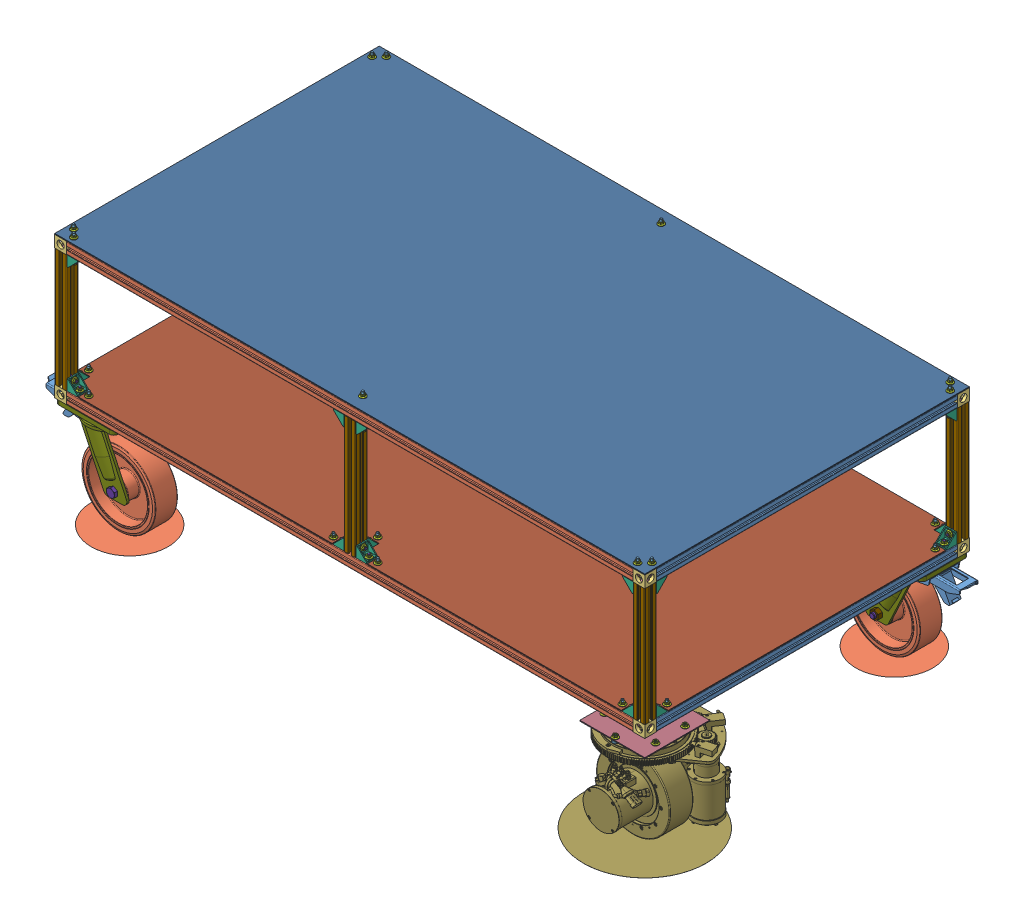
SolidWorks assembly totale, configuration Default. Lengths in mm. (continued)
Components (placement in the parent): (continued)
- body-1: body [Default] at (-233.7628 101.484 2240) size (2000 498.7 1100) (continued)
  - body_skeleton-1: body_skeleton [Default] at (-1.581 -195.357 0) size (2000 480 1100) (continued)
    - Piano_base-2: Piano_base [Default] at (1030.9122 410.7283 -1270) x (1 0 0) z (0 0 -1) size (2000 66.8 1100) (continued)
      - longherone_h-6: longherone_h [Default] at (-560.5014 -11.1801 -790) size (112 40 1043.4)
        - profilato_1020-1: profilato_1020 [Default] at (33.8348 -8.8199 -750) size (40 40 1020)
        - T_BOLT-1: T_BOLT [Default] at (33.8348 -8.8199 276) x (0 -1 0) z (0 0 1) size (19.4 8.5 30.4)
        - T_BOLT-2: T_BOLT [Default] at (33.8348 -8.8199 -756) x (0 -1 0) z (0 0 -1) size (19.4 8.5 30.4)
        - Bracket_40_40_set-2: Bracket_40_40_set [Default] at (-7.7665 -12.3804 -732) x (0 1 0) z (0 0 1) size (38 47.7 51.56)
          - bracket_40_40-1: bracket_40_40 [Default] at (-15.4395 -1.6013 2) size (38 36 36)
          - FLANGE_NUT_M8-3: FLANGE_NUT_M8 [Default] at (3.5605 3.5487 -12.5) size (21 21 8)
          - T_BOLT_short-4: T_BOLT_short [Default] at (3.5605 3.5487 -24) x (-1 0 0) z (0 0 -1) size (19.4 8.5 26.9)
          - FLANGE_NUT_M8-4: FLANGE_NUT_M8 [Default] at (3.5605 -16.1013 7.15) x (0.797177 0 0.603746) z (0 1 0) size (21 21 8)
          - T_BOLT_short-5: T_BOLT_short [Default] at (3.5605 -27.6013 7.15) x (-1 0 0) z (0 -1 0) size (19.4 8.5 26.9)
        - Bracket_40_40_set-3: Bracket_40_40_set [Default] at (75.436 -5.2593 -732) x (0 -1 0) z (0 0 1) size (38 47.7 51.56)
          - bracket_40_40-1: bracket_40_40 [Default] at (-15.4395 -1.6013 2) size (38 36 36)
          - FLANGE_NUT_M8-3: FLANGE_NUT_M8 [Default] at (3.5605 3.5487 -12.5) size (21 21 8)
          - T_BOLT_short-4: T_BOLT_short [Default] at (3.5605 3.5487 -24) x (-1 0 0) z (0 0 -1) size (19.4 8.5 26.9)
          - FLANGE_NUT_M8-4: FLANGE_NUT_M8 [Default] at (3.5605 -16.1013 7.15) x (0.797177 0 0.603746) z (0 1 0) size (21 21 8)
          - T_BOLT_short-5: T_BOLT_short [Default] at (3.5605 -27.6013 7.15) x (-1 0 0) z (0 -1 0) size (19.4 8.5 26.9)
        - Bracket_40_40_set-4: Bracket_40_40_set [Default] at (75.436 -12.3804 252) x (0 1 0) z (0 0 -1) size (38 47.7 51.56)
          - bracket_40_40-1: bracket_40_40 [Default] at (-15.4395 -1.6013 2) size (38 36 36)
          - FLANGE_NUT_M8-3: FLANGE_NUT_M8 [Default] at (3.5605 3.5487 -12.5) size (21 21 8)
          - T_BOLT_short-4: T_BOLT_short [Default] at (3.5605 3.5487 -24) x (-1 0 0) z (0 0 -1) size (19.4 8.5 26.9)
          - FLANGE_NUT_M8-4: FLANGE_NUT_M8 [Default] at (3.5605 -16.1013 7.15) x (0.797177 0 0.603746) z (0 1 0) size (21 21 8)
          - T_BOLT_short-5: T_BOLT_short [Default] at (3.5605 -27.6013 7.15) x (-1 0 0) z (0 -1 0) size (19.4 8.5 26.9)
        - Bracket_40_40_set-5: Bracket_40_40_set [Default] at (-7.7665 -5.2593 252) x (0 -1 0) z (0 0 -1) size (38 47.7 51.56)
          - bracket_40_40-1: bracket_40_40 [Default] at (-15.4395 -1.6013 2) size (38 36 36)
          - FLANGE_NUT_M8-3: FLANGE_NUT_M8 [Default] at (3.5605 3.5487 -12.5) size (21 21 8)
          - T_BOLT_short-4: T_BOLT_short [Default] at (3.5605 3.5487 -24) x (-1 0 0) z (0 0 -1) size (19.4 8.5 26.9)
          - FLANGE_NUT_M8-4: FLANGE_NUT_M8 [Default] at (3.5605 -16.1013 7.15) x (0.797177 0 0.603746) z (0 1 0) size (21 21 8)
          - T_BOLT_short-5: T_BOLT_short [Default] at (3.5605 -27.6013 7.15) x (-1 0 0) z (0 -1 0) size (19.4 8.5 26.9)
      - Bracket_40_40_set-1: Bracket_40_40_set [Default] at (-58 -23.5605 -541.6013) x (0 1 0) z (-1 0 0) size (38 47.7 51.56)
        - bracket_40_40-1: bracket_40_40 [Default] at (-15.4395 -1.6013 2) size (38 36 36)
        - FLANGE_NUT_M8-3: FLANGE_NUT_M8 [Default] at (3.5605 3.5487 -12.5) size (21 21 8)
        - T_BOLT_short-4: T_BOLT_short [Default] at (3.5605 3.5487 -24) x (-1 0 0) z (0 0 -1) size (19.4 8.5 26.9)
        - FLANGE_NUT_M8-4: FLANGE_NUT_M8 [Default] at (3.5605 -16.1013 7.15) x (0.797177 0 0.603746) z (0 1 0) size (21 21 8)
        - T_BOLT_short-5: T_BOLT_short [Default] at (3.5605 -27.6013 7.15) x (-1 0 0) z (0 -1 0) size (19.4 8.5 26.9)
      - Bracket_40_40_set-2: Bracket_40_40_set [Default] at (-1942 -16.4395 -541.6013) x (0 -1 0) z (1 0 0) size (38 47.7 51.56)
        - bracket_40_40-1: bracket_40_40 [Default] at (-15.4395 -1.6013 2) size (38 36 36)
        - FLANGE_NUT_M8-3: FLANGE_NUT_M8 [Default] at (3.5605 3.5487 -12.5) size (21 21 8)
        - T_BOLT_short-4: T_BOLT_short [Default] at (3.5605 3.5487 -24) x (-1 0 0) z (0 0 -1) size (19.4 8.5 26.9)
        - FLANGE_NUT_M8-4: FLANGE_NUT_M8 [Default] at (3.5605 -16.1013 7.15) x (0.797177 0 0.603746) z (0 1 0) size (21 21 8)
        - T_BOLT_short-5: T_BOLT_short [Default] at (3.5605 -27.6013 7.15) x (-1 0 0) z (0 -1 0) size (19.4 8.5 26.9)
      - Bracket_40_40_set-3: Bracket_40_40_set [Default] at (-58 -16.4395 -1518.3987) x (0 -1 0) z (-1 0 0) size (38 47.7 51.56)
        - bracket_40_40-1: bracket_40_40 [Default] at (-15.4395 -1.6013 2) size (38 36 36)
        - FLANGE_NUT_M8-3: FLANGE_NUT_M8 [Default] at (3.5605 3.5487 -12.5) size (21 21 8)
        - T_BOLT_short-4: T_BOLT_short [Default] at (3.5605 3.5487 -24) x (-1 0 0) z (0 0 -1) size (19.4 8.5 26.9)
        - FLANGE_NUT_M8-4: FLANGE_NUT_M8 [Default] at (3.5605 -16.1013 7.15) x (0.797177 0 0.603746) z (0 1 0) size (21 21 8)
        - T_BOLT_short-5: T_BOLT_short [Default] at (3.5605 -27.6013 7.15) x (-1 0 0) z (0 -1 0) size (19.4 8.5 26.9)
      - Bracket_40_40_set-4: Bracket_40_40_set [Default] at (-1938.3987 -16.4395 -1522) x (0 -1 0) z (0 0 1) size (38 47.7 51.56)
        - bracket_40_40-1: bracket_40_40 [Default] at (-15.4395 -1.6013 2) size (38 36 36)
        - FLANGE_NUT_M8-3: FLANGE_NUT_M8 [Default] at (3.5605 3.5487 -12.5) size (21 21 8)
        - T_BOLT_short-4: T_BOLT_short [Default] at (3.5605 3.5487 -24) x (-1 0 0) z (0 0 -1) size (19.4 8.5 26.9)
        - FLANGE_NUT_M8-4: FLANGE_NUT_M8 [Default] at (3.5605 -16.1013 7.15) x (0.797177 0 0.603746) z (0 1 0) size (21 21 8)
        - T_BOLT_short-5: T_BOLT_short [Default] at (3.5605 -27.6013 7.15) x (-1 0 0) z (0 -1 0) size (19.4 8.5 26.9)
  - lastra-1: lastra [Default] at (29.3311 258.3712 -240) x (0 0 1) z (0 1 0) size (1100 2000 3)
  - lastra_down-1: lastra_down [Default] at (29.3311 -184.6288 -240) x (0 0 -1) z (0 -1 0) size (1100 2000 3)
  - T_BOLT-1: T_BOLT [Default] at (-950.6689 -190.6288 -694.75) x (1 0 0) z (0 -1 0) size (19.4 8.5 30.4)
  - T_BOLT-2: T_BOLT [Default] at (-875.4189 -190.6288 -770) x (0 0 1) z (0 -1 0) size (19.4 8.5 30.4)
  - T_BOLT-3: T_BOLT [Default] at (-950.6689 -190.6288 214.75) x (1 0 0) z (0 -1 0) size (19.4 8.5 30.4)
  - T_BOLT-4: T_BOLT [Default] at (-875.4189 -190.6288 290) x (0 0 -1) z (0 -1 0) size (19.4 8.5 30.4)
  - T_BOLT-5: T_BOLT [Default] at (-950.6689 249.3712 -745.75) x (-1 0 0) z (0 -1 0) size (19.4 8.5 30.4)
  - T_BOLT-6: T_BOLT [Default] at (-926.4189 249.3712 -770) x (0 0 -1) z (0 -1 0) size (19.4 8.5 30.4)
  - T_BOLT-7: T_BOLT [Default] at (985.0811 249.3712 -770) x (0 0 -1) z (0 -1 0) size (19.4 8.5 30.4)
  - T_BOLT-8: T_BOLT [Default] at (1009.3311 249.3712 -745.75) x (-1 0 0) z (0 -1 0) size (19.4 8.5 30.4)
  - T_BOLT-9: T_BOLT [Default] at (1009.3311 -190.6288 -694.75) x (-1 0 0) z (0 -1 0) size (19.4 8.5 30.4)
  - T_BOLT-10: T_BOLT [Default] at (934.0811 -190.6288 -770) x (0 0 -1) z (0 -1 0) size (19.4 8.5 30.4)
  - T_BOLT-11: T_BOLT [Default] at (985.0811 249.3712 290) x (0 0 -1) z (0 -1 0) size (19.4 8.5 30.4)
  - T_BOLT-12: T_BOLT [Default] at (1009.3311 249.3712 265.75) x (1 0 0) z (0 -1 0) size (19.4 8.5 30.4)
  - T_BOLT-13: T_BOLT [Default] at (934.0811 -190.6288 290) x (0 0 -1) z (0 -1 0) size (19.4 8.5 30.4)
  - T_BOLT-14: T_BOLT [Default] at (1009.3311 -190.6288 214.75) x (1 0 0) z (0 -1 0) size (19.4 8.5 30.4)
  - T_BOLT-15: T_BOLT [Default] at (-45.9189 -190.6288 290) x (0 0 -1) z (0 -1 0) size (19.4 8.5 30.4)
  - T_BOLT-16: T_BOLT [Default] at (104.5811 -190.6288 290) x (0 0 1) z (0 -1 0) size (19.4 8.5 30.4)
  - T_BOLT-17: T_BOLT [Default] at (29.3311 -190.6288 -694.75) x (-1 0 0) z (0 -1 0) size (19.4 8.5 30.4)
  - T_BOLT-18: T_BOLT [Default] at (-950.6689 249.3712 265.75) x (1 0 0) z (0 -1 0) size (19.4 8.5 30.4)
  - T_BOLT-19: T_BOLT [Default] at (-45.9189 -190.6288 -770) x (0 0 -1) z (0 -1 0) size (19.4 8.5 30.4)
  - T_BOLT-20: T_BOLT [Default] at (104.5811 -190.6288 -770) x (0 0 1) z (0 -1 0) size (19.4 8.5 30.4)
  - T_BOLT-21: T_BOLT [Default] at (29.3311 249.3712 -745.75) x (-1 0 0) z (0 -1 0) size (19.4 8.5 30.4)
  - T_BOLT-22: T_BOLT [Default] at (29.3311 -190.6288 214.75) x (1 0 0) z (0 -1 0) size (19.4 8.5 30.4)
  - T_BOLT-23: T_BOLT [Default] at (29.3311 249.3712 265.75) x (-1 0 0) z (0 -1 0) size (19.4 8.5 30.4)
  - T_BOLT-24: T_BOLT [Default] at (-926.4189 249.3712 290) x (0 0 -1) z (0 -1 0) size (19.4 8.5 30.4)
  - FLANGE_NUT_M8-1: FLANGE_NUT_M8 [Default] at (-950.6689 -181.6288 -694.75) x (1 0 0) z (0 1 0) size (21 21 8)
  - FLANGE_NUT_M8-2: FLANGE_NUT_M8 [Default] at (29.3311 258.3712 -745.75) x (0.999686 0 0.025076) z (0 1 0) size (21 21 8)
  - FLANGE_NUT_M8-3: FLANGE_NUT_M8 [Default] at (29.3311 -181.6288 -694.75) x (1 0 0) z (0 1 0) size (21 21 8)
  - FLANGE_NUT_M8-4: FLANGE_NUT_M8 [Default] at (-875.4189 -181.6288 -770) x (1 0 0) z (0 1 0) size (21 21 8)
  - FLANGE_NUT_M8-5: FLANGE_NUT_M8 [Default] at (-875.4189 -181.6288 290) x (1 0 0) z (0 1 0) size (21 21 8)
  - FLANGE_NUT_M8-6: FLANGE_NUT_M8 [Default] at (-950.6689 -181.6288 214.75) x (1 0 0) z (0 1 0) size (21 21 8)
  - FLANGE_NUT_M8-7: FLANGE_NUT_M8 [Default] at (-45.9189 -181.6288 -770) x (1 0 0) z (0 1 0) size (21 21 8)
  - FLANGE_NUT_M8-8: FLANGE_NUT_M8 [Default] at (-45.9189 -181.6288 290) x (1 0 0) z (0 1 0) size (21 21 8)
  - FLANGE_NUT_M8-9: FLANGE_NUT_M8 [Default] at (-950.6689 258.3712 -745.75) x (1 0 0) z (0 1 0) size (21 21 8)
  - FLANGE_NUT_M8-10: FLANGE_NUT_M8 [Default] at (985.0811 258.3712 -770) x (1 0 0) z (0 1 0) size (21 21 8)
  - FLANGE_NUT_M8-11: FLANGE_NUT_M8 [Default] at (-926.4189 258.3712 290) x (1 0 0) z (0 1 0) size (21 21 8)
  - FLANGE_NUT_M8-12: FLANGE_NUT_M8 [Default] at (1009.3311 258.3712 -745.75) x (1 0 0) z (0 1 0) size (21 21 8)
  - FLANGE_NUT_M8-13: FLANGE_NUT_M8 [Default] at (1009.3311 258.3712 265.75) x (1 0 0) z (0 1 0) size (21 21 8)
  - FLANGE_NUT_M8-14: FLANGE_NUT_M8 [Default] at (934.0811 -181.6288 290) x (1 0 0) z (0 1 0) size (21 21 8)
  - FLANGE_NUT_M8-15: FLANGE_NUT_M8 [Default] at (-926.4189 258.3712 -770) x (1 0 0) z (0 1 0) size (21 21 8)
  - FLANGE_NUT_M8-16: FLANGE_NUT_M8 [Default] at (29.3311 -181.6288 214.75) x (1 0 0) z (0 1 0) size (21 21 8)
  - FLANGE_NUT_M8-17: FLANGE_NUT_M8 [Default] at (934.0811 -181.6288 -770) x (1 0 0) z (0 1 0) size (21 21 8)
  - FLANGE_NUT_M8-18: FLANGE_NUT_M8 [Default] at (104.5811 -181.6288 -770) x (1 0 0) z (0 1 0) size (21 21 8)
  - FLANGE_NUT_M8-19: FLANGE_NUT_M8 [Default] at (1009.3311 -181.6288 214.75) x (1 0 0) z (0 1 0) size (21 21 8)
  - FLANGE_NUT_M8-20: FLANGE_NUT_M8 [Default] at (-950.6689 258.3712 265.75) x (1 0 0) z (0 1 0) size (21 21 8)
  - FLANGE_NUT_M8-21: FLANGE_NUT_M8 [Default] at (985.0811 258.3712 290) x (1 0 0) z (0 1 0) size (21 21 8)
  - FLANGE_NUT_M8-22: FLANGE_NUT_M8 [Default] at (104.5811 -181.6288 290) x (1 0 0) z (0 1 0) size (21 21 8)
  - FLANGE_NUT_M8-23: FLANGE_NUT_M8 [Default] at (1009.3311 -181.6288 -694.75) x (1 0 0) z (0 1 0) size (21 21 8)
  - FLANGE_NUT_M8-24: FLANGE_NUT_M8 [Default] at (29.3311 258.3712 265.75) x (1 0 0) z (0 1 0) size (21 21 8)
- motore+supporto-1: motore+supporto [Default] at (-1125.506 -711.9473 1513.7207) x (-0.999869 -0.016207 0) z (-0.016207 0.999869 -0.000006) size (415.84 415.9 330.44)
  - MR240FRS-AC.stp-1: MR240FRS-AC.stp [Default] at (480.9296 100.5307 -916.9118) size (415.84 415.9 312.91)
  - supporto_motore-2: supporto_motore [Default] at (5.5916 0.2825 575.9688) x (-0.999869 0 -0.016207) z (0.016207 -0.000006 -0.999869) size (220 220 3)
  - distanziale-1: distanziale [Default] at (92.3448 50.2824 567.3735) x (0.92025 -0.391047 0.014919) z (-0.016207 0.000006 0.999869) size (18 18 10)
  - distanziale-2: distanziale [Default] at (-80.8375 -49.7176 564.5668) x (-0.654362 0.756107 -0.010611) z (-0.016207 0.000006 0.999869) size (18 18 10)
  - distanziale-3: distanziale [Default] at (5.7536 -99.7176 565.9707) x (-0.654362 0.756107 -0.010611) z (-0.016207 0.000006 0.999869) size (18 18 10)
  - distanziale-4: distanziale [Default] at (5.5916 100.2825 575.9683) x (-0.701568 -0.712512 -0.011368) z (0.016207 -0.000006 -0.999869) size (18 18 10)
  - distanziale-5: distanziale [Default] at (92.3448 -49.7176 567.374) x (-0.654362 0.756107 -0.010611) z (-0.016207 0.000006 0.999869) size (18 18 10)
  - distanziale-6: distanziale [Default] at (-80.8375 50.2824 564.5663) x (0.92025 -0.391047 0.014919) z (-0.016207 0.000006 0.999869) size (18 18 10)
  - distanziale-7: distanziale [Default] at (-28.6146 -43.7175 588.4163) x (0.316566 0.948557 0.005126) z (0.016207 -0.000006 -0.999869) size (18 18 10)
  - distanziale-8: distanziale [Default] at (49.3751 34.2825 589.6801) x (0.316566 0.948557 0.005126) z (0.016207 -0.000006 -0.999869) size (18 18 10)
  - distanziale-9: distanziale [Default] at (25.1283 -43.7175 589.2875) x (-0.701568 -0.712512 -0.011368) z (0.016207 -0.000006 -0.999869) size (18 18 10)
  - FLANGE_NUT_M8-1: FLANGE_NUT_M8 [Default] at (92.1341 -49.7175 580.3723) x (0.999869 0 0.016207) z (-0.016207 0.000006 0.999869) size (21 21 8)
  - FLANGE_NUT_M8-2: FLANGE_NUT_M8 [Default] at (-81.0482 50.2825 577.5646) x (0.999869 0 0.016207) z (-0.016207 0.000006 0.999869) size (21 21 8)
  - FLANGE_NUT_M8-3: FLANGE_NUT_M8 [Default] at (-81.0482 -49.7175 577.5651) x (0.999869 0 0.016207) z (-0.016207 0.000006 0.999869) size (21 21 8)
  - FLANGE_NUT_M8-4: FLANGE_NUT_M8 [Default] at (5.5429 -99.7175 578.969) x (0.999869 0 0.016207) z (-0.016207 0.000006 0.999869) size (21 21 8)
  - FLANGE_NUT_M8-5: FLANGE_NUT_M8 [Default] at (5.543 100.2825 578.9679) x (0.999869 0 0.016207) z (-0.016207 0.000006 0.999869) size (21 21 8)
  - FLANGE_NUT_M8-6: FLANGE_NUT_M8 [Default] at (92.1342 50.2825 580.3717) x (0.999869 0 0.016207) z (-0.016207 0.000006 0.999869) size (21 21 8)
  - FLANGE_NUT_M8-7: FLANGE_NUT_M8 [Default] at (-28.4039 -43.7175 575.418) x (-0.924292 -0.381392 -0.01498) z (0.016207 -0.000006 -0.999869) size (21 21 8)
  - FLANGE_NUT_M8-8: FLANGE_NUT_M8 [Default] at (25.339 -43.7175 576.2892) x (0.999868 -0.000687 0.016207) z (0.016207 -0.000006 -0.999869) size (21 21 8)
  - FLANGE_NUT_M8-9: FLANGE_NUT_M8 [Default] at (49.5858 34.2825 576.6818) x (-0.924292 -0.381392 -0.01498) z (0.016207 -0.000006 -0.999869) size (21 21 8)
  - slotted countersunk flat head screw_iso-1: slotted countersunk flat head screw_iso [ISO 2009 - M8 x 50 - 38N] at (-80.3351 -49.7178 533.5709) x (-0.016207 0.000006 0.999869) z (-0.999869 -0.000006 -0.016207) size (50 15.8 15.67)
  - slotted countersunk flat head screw_iso-2: slotted countersunk flat head screw_iso [ISO 2009 - M8 x 50 - 38N] at (-3.804 -13.9391 527.2162) size (50 15.8 15.67)
  - slotted countersunk flat head screw_iso-4: slotted countersunk flat head screw_iso [ISO 2009 - M8 x 50 - 38N] at (6.2561 -99.7178 534.9748) x (-0.016207 0.000006 0.999869) z (-0.999869 -0.000006 -0.016207) size (50 15.8 15.67)
  - slotted countersunk flat head screw_iso-5: slotted countersunk flat head screw_iso [ISO 2009 - M8 x 50 - 38N] at (92.8472 -49.7178 536.3781) x (-0.016207 0.000006 0.999869) z (-0.999869 -0.000006 -0.016207) size (50 15.8 15.67)
  - slotted countersunk flat head screw_iso-6: slotted countersunk flat head screw_iso [ISO 2009 - M8 x 50 - 38N] at (-80.3351 50.2822 533.5704) x (-0.016207 0.000006 0.999869) z (-0.999869 -0.000006 -0.016207) size (50 15.8 15.67)
  - slotted countersunk flat head screw_iso-7: slotted countersunk flat head screw_iso [ISO 2009 - M8 x 50 - 38N] at (6.2561 100.2822 534.9737) x (-0.016207 0.000006 0.999869) z (-0.999869 -0.000006 -0.016207) size (50 15.8 15.67)
  - slotted countersunk flat head screw_iso-8: slotted countersunk flat head screw_iso [ISO 2009 - M8 x 50 - 38N] at (92.8473 50.2822 536.3775) x (-0.016207 0.000006 0.999869) z (-0.999869 -0.000006 -0.016207) size (50 15.8 15.67)
  - distanziale-10: distanziale [Default] at (49.3751 -19.4675 589.6804) x (-0.807591 -0.589598 -0.013087) z (0.016207 -0.000006 -0.999869) size (18 18 10)
  - FLANGE_NUT_M8-10: FLANGE_NUT_M8 [Default] at (49.5858 -19.4675 576.6821) x (-0.924292 -0.381392 -0.01498) z (0.016207 -0.000006 -0.999869) size (21 21 8)
- motore+supporto-2: motore+supporto [Default] at (716.6426 -711.9473 2486.2793) x (0.999869 -0.016207 0) z (0.016207 0.999869 0.000006) size (415.84 415.9 330.44)
  - MR240FRS-AC.stp-1: MR240FRS-AC.stp [Default] at (480.9296 100.5307 -916.9118) size (415.84 415.9 312.91)
  - supporto_motore-2: supporto_motore [Default] at (5.5916 0.2825 575.9688) x (-0.999869 0 -0.016207) z (0.016207 -0.000006 -0.999869) size (220 220 3)
  - distanziale-1: distanziale [Default] at (92.3448 50.2824 567.3735) x (0.92025 -0.391047 0.014919) z (-0.016207 0.000006 0.999869) size (18 18 10)
  - distanziale-2: distanziale [Default] at (-80.8375 -49.7176 564.5668) x (-0.654362 0.756107 -0.010611) z (-0.016207 0.000006 0.999869) size (18 18 10)
  - distanziale-3: distanziale [Default] at (5.7536 -99.7176 565.9707) x (-0.654362 0.756107 -0.010611) z (-0.016207 0.000006 0.999869) size (18 18 10)
  - distanziale-4: distanziale [Default] at (5.5916 100.2825 575.9683) x (-0.701568 -0.712512 -0.011368) z (0.016207 -0.000006 -0.999869) size (18 18 10)
  - distanziale-5: distanziale [Default] at (92.3448 -49.7176 567.374) x (-0.654362 0.756107 -0.010611) z (-0.016207 0.000006 0.999869) size (18 18 10)
  - distanziale-6: distanziale [Default] at (-80.8375 50.2824 564.5663) x (0.92025 -0.391047 0.014919) z (-0.016207 0.000006 0.999869) size (18 18 10)
  - distanziale-7: distanziale [Default] at (-28.6146 -43.7175 588.4163) x (0.316566 0.948557 0.005126) z (0.016207 -0.000006 -0.999869) size (18 18 10)
  - distanziale-8: distanziale [Default] at (49.3751 34.2825 589.6801) x (0.316566 0.948557 0.005126) z (0.016207 -0.000006 -0.999869) size (18 18 10)
  - distanziale-9: distanziale [Default] at (25.1283 -43.7175 589.2875) x (-0.701568 -0.712512 -0.011368) z (0.016207 -0.000006 -0.999869) size (18 18 10)
  - FLANGE_NUT_M8-1: FLANGE_NUT_M8 [Default] at (92.1341 -49.7175 580.3723) x (0.999869 0 0.016207) z (-0.016207 0.000006 0.999869) size (21 21 8)
  - FLANGE_NUT_M8-2: FLANGE_NUT_M8 [Default] at (-81.0482 50.2825 577.5646) x (0.999869 0 0.016207) z (-0.016207 0.000006 0.999869) size (21 21 8)
  - FLANGE_NUT_M8-3: FLANGE_NUT_M8 [Default] at (-81.0482 -49.7175 577.5651) x (0.999869 0 0.016207) z (-0.016207 0.000006 0.999869) size (21 21 8)
  - FLANGE_NUT_M8-4: FLANGE_NUT_M8 [Default] at (5.5429 -99.7175 578.969) x (0.999869 0 0.016207) z (-0.016207 0.000006 0.999869) size (21 21 8)
  - FLANGE_NUT_M8-5: FLANGE_NUT_M8 [Default] at (5.543 100.2825 578.9679) x (0.999869 0 0.016207) z (-0.016207 0.000006 0.999869) size (21 21 8)
  - FLANGE_NUT_M8-6: FLANGE_NUT_M8 [Default] at (92.1342 50.2825 580.3717) x (0.999869 0 0.016207) z (-0.016207 0.000006 0.999869) size (21 21 8)
  - FLANGE_NUT_M8-7: FLANGE_NUT_M8 [Default] at (-28.4039 -43.7175 575.418) x (-0.924292 -0.381392 -0.01498) z (0.016207 -0.000006 -0.999869) size (21 21 8)
  - FLANGE_NUT_M8-8: FLANGE_NUT_M8 [Default] at (25.339 -43.7175 576.2892) x (0.999868 -0.000687 0.016207) z (0.016207 -0.000006 -0.999869) size (21 21 8)
  - FLANGE_NUT_M8-9: FLANGE_NUT_M8 [Default] at (49.5858 34.2825 576.6818) x (-0.924292 -0.381392 -0.01498) z (0.016207 -0.000006 -0.999869) size (21 21 8)
  - slotted countersunk flat head screw_iso-1: slotted countersunk flat head screw_iso [ISO 2009 - M8 x 50 - 38N] at (-80.3351 -49.7178 533.5709) x (-0.016207 0.000006 0.999869) z (-0.999869 -0.000006 -0.016207) size (50 15.8 15.67)
  - slotted countersunk flat head screw_iso-2: slotted countersunk flat head screw_iso [ISO 2009 - M8 x 50 - 38N] at (-3.804 -13.9391 527.2162) size (50 15.8 15.67)
  - slotted countersunk flat head screw_iso-4: slotted countersunk flat head screw_iso [ISO 2009 - M8 x 50 - 38N] at (6.2561 -99.7178 534.9748) x (-0.016207 0.000006 0.999869) z (-0.999869 -0.000006 -0.016207) size (50 15.8 15.67)
  - slotted countersunk flat head screw_iso-5: slotted countersunk flat head screw_iso [ISO 2009 - M8 x 50 - 38N] at (92.8472 -49.7178 536.3781) x (-0.016207 0.000006 0.999869) z (-0.999869 -0.000006 -0.016207) size (50 15.8 15.67)
  - slotted countersunk flat head screw_iso-6: slotted countersunk flat head screw_iso [ISO 2009 - M8 x 50 - 38N] at (-80.3351 50.2822 533.5704) x (-0.016207 0.000006 0.999869) z (-0.999869 -0.000006 -0.016207) size (50 15.8 15.67)
  - slotted countersunk flat head screw_iso-7: slotted countersunk flat head screw_iso [ISO 2009 - M8 x 50 - 38N] at (6.2561 100.2822 534.9737) x (-0.016207 0.000006 0.999869) z (-0.999869 -0.000006 -0.016207) size (50 15.8 15.67)
  - slotted countersunk flat head screw_iso-8: slotted countersunk flat head screw_iso [ISO 2009 - M8 x 50 - 38N] at (92.8473 50.2822 536.3775) x (-0.016207 0.000006 0.999869) z (-0.999869 -0.000006 -0.016207) size (50 15.8 15.67)
  - distanziale-10: distanziale [Default] at (49.3751 -19.4675 589.6804) x (-0.807591 -0.589598 -0.013087) z (0.016207 -0.000006 -0.999869) size (18 18 10)
  - FLANGE_NUT_M8-10: FLANGE_NUT_M8 [Default] at (49.5858 -19.4675 576.6821) x (-0.924292 -0.381392 -0.01498) z (0.016207 -0.000006 -0.999869) size (21 21 8)
- T_BOLT-1: T_BOLT [Default] at (-1160.1817 -117.1447 1470) x (0 0 1) z (0 1 0) size (19.4 8.5 30.4)
- T_BOLT-2: T_BOLT [Default] at (-1184.4317 -117.1447 1494.25) x (-1 0 0) z (0 1 0) size (19.4 8.5 30.4)
- T_BOLT-3: T_BOLT [Default] at (-1106.4317 -117.1447 1470) x (0 0 1) z (0 1 0) size (19.4 8.5 30.4)
- T_BOLT-4: T_BOLT [Default] at (-1184.4317 -117.1447 1548) x (1 0 0) z (0 1 0) size (19.4 8.5 30.4)
- T_BOLT-5: T_BOLT [Default] at (751.3183 -117.1447 2530) x (0 0 1) z (0 1 0) size (19.4 8.5 30.4)
- T_BOLT-6: T_BOLT [Default] at (775.5683 -117.1447 2505.75) x (1 0 0) z (0 1 0) size (19.4 8.5 30.4)
- T_BOLT-7: T_BOLT [Default] at (775.5683 -117.1447 2452) x (1 0 0) z (0 1 0) size (19.4 8.5 30.4)
- T_BOLT-8: T_BOLT [Default] at (697.5683 -117.1447 2530) x (0 0 -1) z (0 1 0) size (19.4 8.5 30.4)
- castor_250_manual-1: castor_250_manual [Default] at (-1080.7257 -247.9428 2470) x (-1 0 0) z (0 0 -1) size (393.76 325 260.09)
  - staffa-1: staffa [Default] at (-50.294 -75.2019 0) size (218.5 225 160)
  - Bolt M18-130-1: Bolt M18-130 [Default] at (-50.294 -75.2019 -54) x (0 0 1) z (-1 0 0) size (141.54 31.26 27.08)
  - Nut M18-1: Nut M18 [Default] at (-50.294 -75.2019 69) x (0 0 -1) z (1 0 0) size (15.06 31.22 31.24)
  - freno-1: freno [Default] at (108.036 110.7981 0) size (144.8 81.41 102)
  - Mould-on polyurethane wheels RE.F4-250-RSL.stp-1: Mould-on polyurethane wheels RE.F4-250-RSL.stp [Default] at (-50.294 -75.2019 0) size (260.09 250 260.09)
- castor_250_manual-2: castor_250_manual [Default] at (671.8623 -247.9428 1530) size (393.76 325 260.09)
  - staffa-1: staffa [Default] at (-50.294 -75.2019 0) size (218.5 225 160)
  - Bolt M18-130-1: Bolt M18-130 [Default] at (-50.294 -75.2019 -54) x (0 0 1) z (-1 0 0) size (141.54 31.26 27.08)
  - Nut M18-1: Nut M18 [Default] at (-50.294 -75.2019 69) x (0 0 -1) z (1 0 0) size (15.06 31.22 31.24)
  - freno-1: freno [Default] at (108.036 110.7981 0) size (144.8 81.41 102)
  - Mould-on polyurethane wheels RE.F4-250-RSL.stp-1: Mould-on polyurethane wheels RE.F4-250-RSL.stp [Default] at (-50.294 -75.2019 0) size (260.09 250 260.09)
Mates (geometry in assembly coordinates):
- Coincidente3: coincident anti-aligned: plane of body-1/body_skeleton-1/Piano_base-1/cubic_joint_screws-2/cubic_joint_3-1 through (-1184.4317 -103.1447 1490) normal (0 0 1); plane of T_BOLT-2 through (-1184.4317 -117.1447 1490) normal (0 0 -1)
- Coincidente4: coincident anti-aligned: plane of body-1/body_skeleton-1/Piano_base-1/profilato_1020-2 through (-1189.4317 -121.6447 1490) normal (1 0 0); plane of T_BOLT-2 through (-1189.4317 -117.1447 1490) normal (-1 0 0)
- Coincidente5: coincident anti-aligned: plane of body-1/body_skeleton-1/Piano_base-1/profilato_1920-1 through (-1164.4317 -121.6447 1475) normal (0 0 -1); plane of T_BOLT-1 through (-1164.4317 -117.1447 1475) normal (0 0 1)
- Coincidente6: coincident anti-aligned: plane of body-1/body_skeleton-1/Piano_base-1/cubic_joint_screws-2/cubic_joint_3-1 through (-1164.4317 -103.1447 1470) normal (1 0 0); plane of T_BOLT-1 through (-1164.4317 -117.1447 1470) normal (-1 0 0)
- Coincidente7: coincident anti-aligned: plane of body-1/body_skeleton-1/Piano_base-1/profilato_1920-1 through (-1164.4317 -121.6447 1475) normal (0 0 -1); plane of T_BOLT-3 through (-1110.6817 -117.1447 1475) normal (0 0 1)
- Coincidente8: coincident aligned: plane of T_BOLT-1 through (-1164.4317 -121.8447 1465.75) normal (0 -1 0); plane of T_BOLT-3 through (-1110.6817 -121.8447 1465.75) normal (0 -1 0)
- Coincidente9: coincident aligned: plane of T_BOLT-1 through (-1164.4317 -121.8447 1465.75) normal (0 -1 0); plane of T_BOLT-2 through (-1180.1817 -121.8447 1490) normal (0 -1 0)
- Coincidente10: coincident anti-aligned: plane of body-1/body_skeleton-1/Piano_base-1/profilato_1020-2 through (-1179.4317 -117.1447 1490) normal (0 1 0); plane of T_BOLT-2 through (-1179.4317 -117.1447 1490) normal (0 -1 0)
- Concentrico1: concentric anti-aligned: cylinder of motore+supporto-1/distanziale-9 through (-1160.1817 -133.1447 1470) axis (0 1 0) radius 4; cylinder of T_BOLT-1 through (-1160.1817 -120.6447 1470) axis (0 -1 0) radius 4
- Coincidente11: coincident aligned: plane of T_BOLT-2 through (-1180.1817 -121.8447 1490) normal (0 -1 0); plane of T_BOLT-4 through (-1188.6817 -121.8447 1552.25) normal (0 -1 0)
- Coincidente12: coincident anti-aligned: plane of body-1/body_skeleton-1/Piano_base-1/profilato_1020-2 through (-1179.4317 -121.6447 1490) normal (-1 0 0); plane of T_BOLT-4 through (-1179.4317 -117.1447 1552.25) normal (1 0 0)
- Concentrico2: concentric anti-aligned: cylinder of motore+supporto-1/distanziale-10 through (-1184.4317 -133.1447 1494.25) axis (0 1 0) radius 4; cylinder of T_BOLT-2 through (-1184.4317 -120.6447 1494.25) axis (0 -1 0) radius 4
- Concentrico3: concentric anti-aligned: cylinder of motore+supporto-1/distanziale-8 through (-1184.4317 -133.1447 1548) axis (0 1 0) radius 4; cylinder of T_BOLT-4 through (-1184.4317 -120.6447 1548) axis (0 -1 0) radius 4
- Concentrico4: concentric anti-aligned: cylinder of motore+supporto-1/distanziale-7 through (-1106.4317 -133.1447 1470) axis (0 1 0) radius 4; cylinder of T_BOLT-3 through (-1106.4317 -120.6447 1470) axis (0 -1 0) radius 4
- Coincidente13: coincident anti-aligned: plane of body-1/body_skeleton-1/Piano_base-1/profilato_1920-1 through (-1164.4317 -123.1447 1453) normal (0 -1 0); plane of motore+supporto-1/distanziale-9 through (-1160.1817 -123.1447 1470) normal (0 1 0)
- Coincidente14: coincident anti-aligned: plane of body-1/body_skeleton-1/Piano_base-1/profilato_1920-2 through (-1164.4317 -117.1447 2535) normal (0 0 -1); plane of T_BOLT-5 through (747.0683 -117.1447 2535) normal (0 0 1)
- Coincidente15: coincident anti-aligned: plane of body-1/body_skeleton-1/Piano_base-1/cubic_joint_screws-3/cubic_joint_3-1 through (755.5683 -103.1447 2530) normal (-1 0 0); plane of T_BOLT-5 through (755.5683 -117.1447 2530) normal (1 0 0)
- Coincidente16: coincident anti-aligned: plane of body-1/body_skeleton-1/Piano_base-1/cubic_joint_screws-3/cubic_joint_3-1 through (775.5683 -103.1447 2510) normal (0 0 -1); plane of T_BOLT-6 through (775.5683 -117.1447 2510) normal (0 0 1)
- Coincidente17: coincident anti-aligned: plane of body-1/body_skeleton-1/Piano_base-1/profilato_1020-1 through (770.5683 -117.1447 2510) normal (1 0 0); plane of T_BOLT-6 through (770.5683 -120.6447 2510) normal (-1 0 0)
- Coincidente18: coincident aligned: plane of T_BOLT-5 through (747.0683 -121.8447 2525.75) normal (0 -1 0); plane of T_BOLT-6 through (771.3183 -121.8447 2510) normal (0 -1 0)
- Coincidente19: coincident aligned: plane of T_BOLT-6 through (771.3183 -121.8447 2510) normal (0 -1 0); plane of T_BOLT-7 through (771.3183 -121.8447 2456.25) normal (0 -1 0)
- Coincidente20: coincident anti-aligned: plane of body-1/body_skeleton-1/Piano_base-1/profilato_1020-1 through (770.5683 -117.1447 2510) normal (1 0 0); plane of T_BOLT-7 through (770.5683 -120.6447 2456.25) normal (-1 0 0)
- Coincidente21: coincident aligned: plane of T_BOLT-5 through (747.0683 -121.8447 2525.75) normal (0 -1 0); plane of T_BOLT-8 through (701.8183 -121.8447 2534.25) normal (0 -1 0)
- Coincidente22: coincident anti-aligned: plane of body-1/body_skeleton-1/Piano_base-1/profilato_1920-2 through (-1164.4317 -117.1447 2535) normal (0 0 -1); plane of T_BOLT-8 through (701.8183 -120.6447 2535) normal (0 0 1)
- Coincidente23: coincident aligned: plane of T_BOLT-3 through (-1110.6817 -121.8447 1465.75) normal (0 -1 0); plane of T_BOLT-5 through (747.0683 -121.8447 2525.75) normal (0 -1 0)
- Concentrico5: concentric anti-aligned: cylinder of motore+supporto-2/distanziale-10 through (775.5683 -133.1447 2505.75) axis (0 1 0) radius 4; cylinder of T_BOLT-6 through (775.5683 -120.6447 2505.75) axis (0 -1 0) radius 4
- Concentrico6: concentric anti-aligned: cylinder of motore+supporto-2/distanziale-9 through (751.3183 -133.1447 2530) axis (0 1 0) radius 4; cylinder of T_BOLT-5 through (751.3183 -120.6447 2530) axis (0 -1 0) radius 4
- Concentrico7: concentric anti-aligned: cylinder of motore+supporto-2/distanziale-7 through (697.5683 -133.1447 2530) axis (0 1 0) radius 4; cylinder of T_BOLT-8 through (697.5683 -120.6447 2530) axis (0 -1 0) radius 4
- Concentrico9: concentric anti-aligned: cylinder of motore+supporto-2/distanziale-8 through (775.5683 -133.1447 2452) axis (0 1 0) radius 4; cylinder of T_BOLT-7 through (775.5683 -120.6447 2452) axis (0 -1 0) radius 4
- Coincidente24: coincident anti-aligned: plane of body-1/body_skeleton-1/Piano_base-1/profilato_1020-1 through (781.3683 -123.1447 2510) normal (0 -1 0); plane of motore+supporto-2/distanziale-10 through (775.5683 -123.1447 2505.75) normal (0 1 0)
- Coincidente25: coincident aligned: plane of body-1/body_skeleton-1/Piano_base-1/cubic_joint_screws-4/cubic_joint_3-1 through (-1204.4317 -103.1447 2530) normal (-1 0 0); plane of castor_250_manual-1/staffa-1 through (-1204.4317 -137.1447 2405) normal (-1 0 0)
- Coincidente26: coincident aligned: plane of body-1/body_skeleton-1/Piano_base-1/cubic_joint_screws-4/cubic_joint_3-1 through (-1184.4317 -103.1447 2550) normal (0 0 1); plane of castor_250_manual-1/staffa-1 through (-1189.4317 -137.1447 2550) normal (0 0 1)
- Coincidente27: coincident anti-aligned: plane of body-1/body_skeleton-1/Piano_base-1/cubic_joint_screws-4/cubic_joint_3-1 through (-1184.4317 -123.1447 2530) normal (0 -1 0); plane of castor_250_manual-1/staffa-1 through (-1019.4317 -123.1447 2535) normal (0 1 0)
- Coincidente29: coincident: plane of body-1/body_skeleton-1/Piano_base-1/cubic_joint_screws-1/cubic_joint_3-1 through (775.5683 -103.1447 1450) normal (0 0 -1); plane of castor_250_manual-2/staffa-1 through (780.5683 -193.742 1450) normal (0 0 -1)
- Coincidente31: coincident: plane of body-1/body_skeleton-1/Piano_base-1/cubic_joint_screws-1/cubic_joint_3-1 through (795.5683 -103.1447 1470) normal (1 0 0); plane of castor_250_manual-2/staffa-1 through (795.5683 -193.742 1595) normal (1 0 0)
- Coincidente32: coincident anti-aligned: plane of body-1/body_skeleton-1/Piano_base-1/cubic_joint_screws-1/cubic_joint_3-1 through (775.5683 -123.1447 1470) normal (0 -1 0); plane of castor_250_manual-2/staffa-1 through (610.5683 -179.742 1465) normal (0 1 0)
